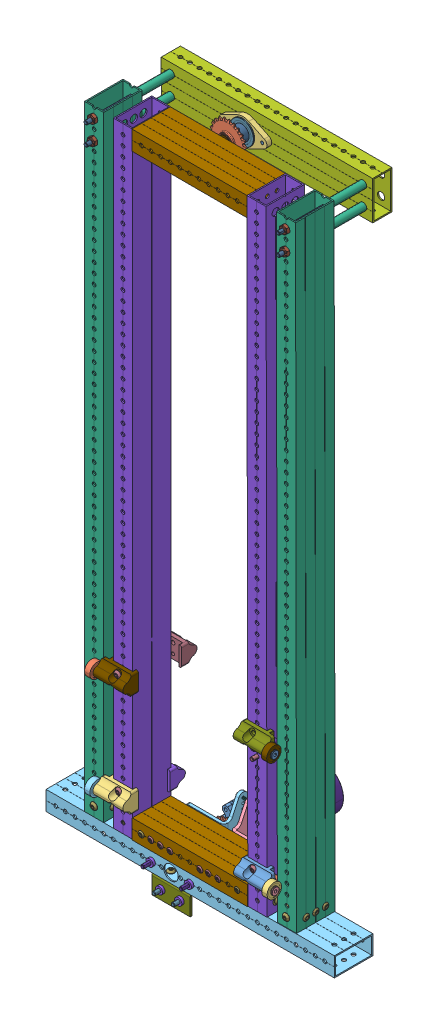
SolidWorks assembly WCP - GreyT Elevator (Cascade, 1 Stage).step, configuration Default. Lengths in mm.
Overall size (381 869.61 219.47).
186 component instances, 76 part files, 114 mates.
Components (placement in the parent):
- WCP-0323 - Elevator Clamping Block^WCP - GreyT Elevator (Cascade, 1 Stage).step-1: WCP-0323 - Elevator Clamping Block^WCP - GreyT Elevator (Cascade, 1 Stage).step [Default] at (101.6635 57.15 25.4) x (0 0 -1) z (1 0 0) size (29.22 25.41 49.35) (virtual)
  - WCP-0323-001 Rev2(7)^WCP-0323 - Elevator Clamping Block_WCP - GreyT Elevator (Cascade, 1 Stage).step-1: WCP-0323-001 Rev2(7)^WCP-0323 - Elevator Clamping Block_WCP - GreyT Elevator (Cascade, 1 Stage).step [Default] at origin size (20.38 25.41 40.49) (virtual)
  - WCP-0498 Rev1(7)^WCP-0323 - Elevator Clamping Block_WCP - GreyT Elevator (Cascade, 1 Stage).step-1: WCP-0498 Rev1(7)^WCP-0323 - Elevator Clamping Block_WCP - GreyT Elevator (Cascade, 1 Stage).step [Default] at (2.254 0 6.7) x (0 0.307359 0.951594) z (-1 0 0) size (12 12 4) (virtual)
  - WCP-0212_0_250_radial_bearing(7)^WCP-0323 - Elevator Clamping Block_WCP - GreyT Elevator (Cascade, 1 Stage).step-1: WCP-0212_0_250_radial_bearing(7)^WCP-0323 - Elevator Clamping Block_WCP - GreyT Elevator (Cascade, 1 Stage).step [Default] at (-9.525 0 15.4781) size (19.05 19.05 7.14) (virtual)
  - WCP-0473 Rev1(7)^WCP-0323 - Elevator Clamping Block_WCP - GreyT Elevator (Cascade, 1 Stage).step-1: WCP-0473 Rev1(7)^WCP-0323 - Elevator Clamping Block_WCP - GreyT Elevator (Cascade, 1 Stage).step [Default] at (-9.525 0 10.4394) x (-0.082744 -0.996571 0) z (-0.996571 0.082744 0) size (9.53 20.65 9.53) (virtual)
  - #8-32 x .25L BHCS(7)^WCP-0323 - Elevator Clamping Block_WCP - GreyT Elevator (Cascade, 1 Stage).step-1: #8-32 x .25L BHCS(7)^WCP-0323 - Elevator Clamping Block_WCP - GreyT Elevator (Cascade, 1 Stage).step [Default] at (6.7178 0 6.7) x (0 -0.337236 -0.94142) z (1 0 0) size (10.28 8 12.02) (virtual)
- WCP-0323 - Elevator Clamping Block-1^WCP - GreyT Elevator (Cascade, 1 Stage).step-1: WCP-0323 - Elevator Clamping Block-1^WCP - GreyT Elevator (Cascade, 1 Stage).step [Default] at (101.6635 57.15 -25.4) x (0 0 1) z (1 0 0) size (29.22 25.41 49.35) (virtual)
  - WCP-0323-001 Rev2(4)^WCP-0323 - Elevator Clamping Block-1_WCP - GreyT Elevator (Cascade, 1 Stage).step-1: WCP-0323-001 Rev2(4)^WCP-0323 - Elevator Clamping Block-1_WCP - GreyT Elevator (Cascade, 1 Stage).step [Default] at origin size (20.38 25.41 40.49) (virtual)
  - WCP-0498 Rev1(4)^WCP-0323 - Elevator Clamping Block-1_WCP - GreyT Elevator (Cascade, 1 Stage).step-1: WCP-0498 Rev1(4)^WCP-0323 - Elevator Clamping Block-1_WCP - GreyT Elevator (Cascade, 1 Stage).step [Default] at (2.254 0 6.7) x (0 0.307359 0.951594) z (-1 0 0) size (12 12 4) (virtual)
  - WCP-0212_0_250_radial_bearing(4)^WCP-0323 - Elevator Clamping Block-1_WCP - GreyT Elevator (Cascade, 1 Stage).step-1: WCP-0212_0_250_radial_bearing(4)^WCP-0323 - Elevator Clamping Block-1_WCP - GreyT Elevator (Cascade, 1 Stage).step [Default] at (-9.525 0 15.4781) size (19.05 19.05 7.14) (virtual)
  - WCP-0473 Rev1(4)^WCP-0323 - Elevator Clamping Block-1_WCP - GreyT Elevator (Cascade, 1 Stage).step-1: WCP-0473 Rev1(4)^WCP-0323 - Elevator Clamping Block-1_WCP - GreyT Elevator (Cascade, 1 Stage).step [Default] at (-9.525 0 10.4394) x (-0.082744 -0.996571 0) z (-0.996571 0.082744 0) size (9.53 20.65 9.53) (virtual)
  - #8-32 x .25L BHCS(4)^WCP-0323 - Elevator Clamping Block-1_WCP - GreyT Elevator (Cascade, 1 Stage).step-1: #8-32 x .25L BHCS(4)^WCP-0323 - Elevator Clamping Block-1_WCP - GreyT Elevator (Cascade, 1 Stage).step [Default] at (6.7178 0 6.7) x (0 -0.337236 -0.94142) z (1 0 0) size (10.28 8 12.02) (virtual)
- WCP-0323 - Elevator Clamping Block-2^WCP - GreyT Elevator (Cascade, 1 Stage).step-1: WCP-0323 - Elevator Clamping Block-2^WCP - GreyT Elevator (Cascade, 1 Stage).step [Default] at (101.6635 196.85 -25.4) x (0 0 1) z (1 0 0) size (29.22 25.41 49.35) (virtual)
  - WCP-0323-001 Rev2^WCP-0323 - Elevator Clamping Block-2_WCP - GreyT Elevator (Cascade, 1 Stage).step-1: WCP-0323-001 Rev2^WCP-0323 - Elevator Clamping Block-2_WCP - GreyT Elevator (Cascade, 1 Stage).step [Default] at origin size (20.38 25.41 40.49) (virtual)
  - WCP-0498 Rev1^WCP-0323 - Elevator Clamping Block-2_WCP - GreyT Elevator (Cascade, 1 Stage).step-1: WCP-0498 Rev1^WCP-0323 - Elevator Clamping Block-2_WCP - GreyT Elevator (Cascade, 1 Stage).step [Default] at (2.254 0 6.7) x (0 0.307359 0.951594) z (-1 0 0) size (12 12 4) (virtual)
  - WCP-0212_0_250_radial_bearing^WCP-0323 - Elevator Clamping Block-2_WCP - GreyT Elevator (Cascade, 1 Stage).step-1: WCP-0212_0_250_radial_bearing^WCP-0323 - Elevator Clamping Block-2_WCP - GreyT Elevator (Cascade, 1 Stage).step [Default] at (-9.525 0 15.4781) size (19.05 19.05 7.14) (virtual)
  - WCP-0473 Rev1^WCP-0323 - Elevator Clamping Block-2_WCP - GreyT Elevator (Cascade, 1 Stage).step-1: WCP-0473 Rev1^WCP-0323 - Elevator Clamping Block-2_WCP - GreyT Elevator (Cascade, 1 Stage).step [Default] at (-9.525 0 10.4394) x (-0.082744 -0.996571 0) z (-0.996571 0.082744 0) size (9.53 20.65 9.53) (virtual)
  - #8-32 x .25L BHCS^WCP-0323 - Elevator Clamping Block-2_WCP - GreyT Elevator (Cascade, 1 Stage).step-1: #8-32 x .25L BHCS^WCP-0323 - Elevator Clamping Block-2_WCP - GreyT Elevator (Cascade, 1 Stage).step [Default] at (6.7178 0 6.7) x (0 -0.337236 -0.94142) z (1 0 0) size (10.28 8 12.02) (virtual)
- WCP-0323 - Elevator Clamping Block-3^WCP - GreyT Elevator (Cascade, 1 Stage).step-1: WCP-0323 - Elevator Clamping Block-3^WCP - GreyT Elevator (Cascade, 1 Stage).step [Default] at (102.2013 214.1019 26.4322) x (0.002419 0.000009 -0.999997) z (0.999996 0.001569 0.002419) size (29.22 25.41 49.35) (virtual)
  - WCP-0323-001 Rev2(8)^WCP-0323 - Elevator Clamping Block-3_WCP - GreyT Elevator (Cascade, 1 Stage).step-1: WCP-0323-001 Rev2(8)^WCP-0323 - Elevator Clamping Block-3_WCP - GreyT Elevator (Cascade, 1 Stage).step [Default] at origin size (20.38 25.41 40.49) (virtual)
  - WCP-0498 Rev1(8)^WCP-0323 - Elevator Clamping Block-3_WCP - GreyT Elevator (Cascade, 1 Stage).step-1: WCP-0498 Rev1(8)^WCP-0323 - Elevator Clamping Block-3_WCP - GreyT Elevator (Cascade, 1 Stage).step [Default] at (2.254 0 6.7) x (0 0.307359 0.951594) z (-1 0 0) size (12 12 4) (virtual)
  - WCP-0212_0_250_radial_bearing(8)^WCP-0323 - Elevator Clamping Block-3_WCP - GreyT Elevator (Cascade, 1 Stage).step-1: WCP-0212_0_250_radial_bearing(8)^WCP-0323 - Elevator Clamping Block-3_WCP - GreyT Elevator (Cascade, 1 Stage).step [Default] at (-9.525 0 15.4781) size (19.05 19.05 7.14) (virtual)
  - WCP-0473 Rev1(8)^WCP-0323 - Elevator Clamping Block-3_WCP - GreyT Elevator (Cascade, 1 Stage).step-1: WCP-0473 Rev1(8)^WCP-0323 - Elevator Clamping Block-3_WCP - GreyT Elevator (Cascade, 1 Stage).step [Default] at (-9.525 0 10.4394) x (-0.082744 -0.996571 0) z (-0.996571 0.082744 0) size (9.53 20.65 9.53) (virtual)
  - #8-32 x .25L BHCS(8)^WCP-0323 - Elevator Clamping Block-3_WCP - GreyT Elevator (Cascade, 1 Stage).step-1: #8-32 x .25L BHCS(8)^WCP-0323 - Elevator Clamping Block-3_WCP - GreyT Elevator (Cascade, 1 Stage).step [Default] at (6.7178 0 6.7) x (0 -0.337236 -0.94142) z (1 0 0) size (10.28 8 12.02) (virtual)
- WCP-0323 - Elevator Clamping Block-4^WCP - GreyT Elevator (Cascade, 1 Stage).step-1: WCP-0323 - Elevator Clamping Block-4^WCP - GreyT Elevator (Cascade, 1 Stage).step [Default] at (-101.6635 57.15 25.4) x (0 0 -1) z (-1 0 0) size (29.22 25.41 49.35) (virtual)
  - WCP-0323-001 Rev2(5)^WCP-0323 - Elevator Clamping Block-4_WCP - GreyT Elevator (Cascade, 1 Stage).step-1: WCP-0323-001 Rev2(5)^WCP-0323 - Elevator Clamping Block-4_WCP - GreyT Elevator (Cascade, 1 Stage).step [Default] at origin size (20.38 25.41 40.49) (virtual)
  - WCP-0498 Rev1(5)^WCP-0323 - Elevator Clamping Block-4_WCP - GreyT Elevator (Cascade, 1 Stage).step-1: WCP-0498 Rev1(5)^WCP-0323 - Elevator Clamping Block-4_WCP - GreyT Elevator (Cascade, 1 Stage).step [Default] at (2.254 0 6.7) x (0 0.307359 0.951594) z (-1 0 0) size (12 12 4) (virtual)
  - WCP-0212_0_250_radial_bearing(5)^WCP-0323 - Elevator Clamping Block-4_WCP - GreyT Elevator (Cascade, 1 Stage).step-1: WCP-0212_0_250_radial_bearing(5)^WCP-0323 - Elevator Clamping Block-4_WCP - GreyT Elevator (Cascade, 1 Stage).step [Default] at (-9.525 0 15.4781) size (19.05 19.05 7.14) (virtual)
  - WCP-0473 Rev1(5)^WCP-0323 - Elevator Clamping Block-4_WCP - GreyT Elevator (Cascade, 1 Stage).step-1: WCP-0473 Rev1(5)^WCP-0323 - Elevator Clamping Block-4_WCP - GreyT Elevator (Cascade, 1 Stage).step [Default] at (-9.525 0 10.4394) x (-0.082744 -0.996571 0) z (-0.996571 0.082744 0) size (9.53 20.65 9.53) (virtual)
  - #8-32 x .25L BHCS(5)^WCP-0323 - Elevator Clamping Block-4_WCP - GreyT Elevator (Cascade, 1 Stage).step-1: #8-32 x .25L BHCS(5)^WCP-0323 - Elevator Clamping Block-4_WCP - GreyT Elevator (Cascade, 1 Stage).step [Default] at (6.7178 0 6.7) x (0 -0.337236 -0.94142) z (1 0 0) size (10.28 8 12.02) (virtual)
- WCP-0323 - Elevator Clamping Block-5^WCP - GreyT Elevator (Cascade, 1 Stage).step-1: WCP-0323 - Elevator Clamping Block-5^WCP - GreyT Elevator (Cascade, 1 Stage).step [Default] at (-101.6635 57.15 -25.4) x (0 0 1) z (-1 0 0) size (29.22 25.41 49.35) (virtual)
  - WCP-0323-001 Rev2(2)^WCP-0323 - Elevator Clamping Block-5_WCP - GreyT Elevator (Cascade, 1 Stage).step-1: WCP-0323-001 Rev2(2)^WCP-0323 - Elevator Clamping Block-5_WCP - GreyT Elevator (Cascade, 1 Stage).step [Default] at origin size (20.38 25.41 40.49) (virtual)
  - WCP-0498 Rev1(2)^WCP-0323 - Elevator Clamping Block-5_WCP - GreyT Elevator (Cascade, 1 Stage).step-1: WCP-0498 Rev1(2)^WCP-0323 - Elevator Clamping Block-5_WCP - GreyT Elevator (Cascade, 1 Stage).step [Default] at (2.254 0 6.7) x (0 0.307359 0.951594) z (-1 0 0) size (12 12 4) (virtual)
  - WCP-0212_0_250_radial_bearing(2)^WCP-0323 - Elevator Clamping Block-5_WCP - GreyT Elevator (Cascade, 1 Stage).step-1: WCP-0212_0_250_radial_bearing(2)^WCP-0323 - Elevator Clamping Block-5_WCP - GreyT Elevator (Cascade, 1 Stage).step [Default] at (-9.525 0 15.4781) size (19.05 19.05 7.14) (virtual)
  - WCP-0473 Rev1(2)^WCP-0323 - Elevator Clamping Block-5_WCP - GreyT Elevator (Cascade, 1 Stage).step-1: WCP-0473 Rev1(2)^WCP-0323 - Elevator Clamping Block-5_WCP - GreyT Elevator (Cascade, 1 Stage).step [Default] at (-9.525 0 10.4394) x (-0.082744 -0.996571 0) z (-0.996571 0.082744 0) size (9.53 20.65 9.53) (virtual)
  - #8-32 x .25L BHCS(2)^WCP-0323 - Elevator Clamping Block-5_WCP - GreyT Elevator (Cascade, 1 Stage).step-1: #8-32 x .25L BHCS(2)^WCP-0323 - Elevator Clamping Block-5_WCP - GreyT Elevator (Cascade, 1 Stage).step [Default] at (6.7178 0 6.7) x (0 -0.337236 -0.94142) z (1 0 0) size (10.28 8 12.02) (virtual)
- WCP-0323 - Elevator Clamping Block-6^WCP - GreyT Elevator (Cascade, 1 Stage).step-1: WCP-0323 - Elevator Clamping Block-6^WCP - GreyT Elevator (Cascade, 1 Stage).step [Default] at (-101.6 192.0731 -40.688) x (0 0 1) z (-1 0 0) size (29.22 25.41 49.35) (virtual)
  - WCP-0323-001 Rev2(3)^WCP-0323 - Elevator Clamping Block-6_WCP - GreyT Elevator (Cascade, 1 Stage).step-1: WCP-0323-001 Rev2(3)^WCP-0323 - Elevator Clamping Block-6_WCP - GreyT Elevator (Cascade, 1 Stage).step [Default] at origin size (20.38 25.41 40.49) (virtual)
  - WCP-0498 Rev1(3)^WCP-0323 - Elevator Clamping Block-6_WCP - GreyT Elevator (Cascade, 1 Stage).step-1: WCP-0498 Rev1(3)^WCP-0323 - Elevator Clamping Block-6_WCP - GreyT Elevator (Cascade, 1 Stage).step [Default] at (2.254 0 6.7) x (0 0.307359 0.951594) z (-1 0 0) size (12 12 4) (virtual)
  - WCP-0212_0_250_radial_bearing(3)^WCP-0323 - Elevator Clamping Block-6_WCP - GreyT Elevator (Cascade, 1 Stage).step-1: WCP-0212_0_250_radial_bearing(3)^WCP-0323 - Elevator Clamping Block-6_WCP - GreyT Elevator (Cascade, 1 Stage).step [Default] at (-9.525 0 15.4781) size (19.05 19.05 7.14) (virtual)
  - WCP-0473 Rev1(3)^WCP-0323 - Elevator Clamping Block-6_WCP - GreyT Elevator (Cascade, 1 Stage).step-1: WCP-0473 Rev1(3)^WCP-0323 - Elevator Clamping Block-6_WCP - GreyT Elevator (Cascade, 1 Stage).step [Default] at (-9.525 0 10.4394) x (-0.082744 -0.996571 0) z (-0.996571 0.082744 0) size (9.53 20.65 9.53) (virtual)
  - #8-32 x .25L BHCS(3)^WCP-0323 - Elevator Clamping Block-6_WCP - GreyT Elevator (Cascade, 1 Stage).step-1: #8-32 x .25L BHCS(3)^WCP-0323 - Elevator Clamping Block-6_WCP - GreyT Elevator (Cascade, 1 Stage).step [Default] at (6.7178 0 6.7) x (0 -0.337236 -0.94142) z (1 0 0) size (10.28 8 12.02) (virtual)
- WCP-0323 - Elevator Clamping Block-7^WCP - GreyT Elevator (Cascade, 1 Stage).step-1: WCP-0323 - Elevator Clamping Block-7^WCP - GreyT Elevator (Cascade, 1 Stage).step [Default] at (-101.6 192.0731 25.4) x (0 0 -1) z (-1 0 0) size (29.22 25.41 49.35) (virtual)
  - WCP-0323-001 Rev2(6)^WCP-0323 - Elevator Clamping Block-7_WCP - GreyT Elevator (Cascade, 1 Stage).step-1: WCP-0323-001 Rev2(6)^WCP-0323 - Elevator Clamping Block-7_WCP - GreyT Elevator (Cascade, 1 Stage).step [Default] at origin size (20.38 25.41 40.49) (virtual)
  - WCP-0498 Rev1(6)^WCP-0323 - Elevator Clamping Block-7_WCP - GreyT Elevator (Cascade, 1 Stage).step-1: WCP-0498 Rev1(6)^WCP-0323 - Elevator Clamping Block-7_WCP - GreyT Elevator (Cascade, 1 Stage).step [Default] at (2.254 0 6.7) x (0 0.307359 0.951594) z (-1 0 0) size (12 12 4) (virtual)
  - WCP-0212_0_250_radial_bearing(6)^WCP-0323 - Elevator Clamping Block-7_WCP - GreyT Elevator (Cascade, 1 Stage).step-1: WCP-0212_0_250_radial_bearing(6)^WCP-0323 - Elevator Clamping Block-7_WCP - GreyT Elevator (Cascade, 1 Stage).step [Default] at (-9.525 0 15.4781) size (19.05 19.05 7.14) (virtual)
  - WCP-0473 Rev1(6)^WCP-0323 - Elevator Clamping Block-7_WCP - GreyT Elevator (Cascade, 1 Stage).step-1: WCP-0473 Rev1(6)^WCP-0323 - Elevator Clamping Block-7_WCP - GreyT Elevator (Cascade, 1 Stage).step [Default] at (-9.525 0 10.4394) x (-0.082744 -0.996571 0) z (-0.996571 0.082744 0) size (9.53 20.65 9.53) (virtual)
  - #8-32 x .25L BHCS(6)^WCP-0323 - Elevator Clamping Block-7_WCP - GreyT Elevator (Cascade, 1 Stage).step-1: #8-32 x .25L BHCS(6)^WCP-0323 - Elevator Clamping Block-7_WCP - GreyT Elevator (Cascade, 1 Stage).step [Default] at (6.7178 0 6.7) x (0 -0.337236 -0.94142) z (1 0 0) size (10.28 8 12.02) (virtual)
- WCP-EX-0018-001^WCP - GreyT Elevator (Cascade, 1 Stage).step-1: WCP-EX-0018-001^WCP - GreyT Elevator (Cascade, 1 Stage).step [Default] x (1 0 0) z (0 -1 0) size (381 50.8 25.4) (virtual)
- WCP-EX-0018-005^WCP - GreyT Elevator (Cascade, 1 Stage).step-1: WCP-EX-0018-005^WCP - GreyT Elevator (Cascade, 1 Stage).step [Default] at (127.0437 610.2494 0.0748) x (0.001569 -0.999999 -0.000005) z (0.999996 0.001569 0.002419) size (812.8 50.8 25.4) (virtual)
- WCP-EX-0018-002^WCP - GreyT Elevator (Cascade, 1 Stage).step-1: WCP-EX-0018-002^WCP - GreyT Elevator (Cascade, 1 Stage).step [Default] at (0.0319 800.4229 -88.6828) x (0.999997 0.002542 0) z (0 0 1) size (279.4 50.8 25.4) (virtual)
- WCP-EX-0018-003^WCP - GreyT Elevator (Cascade, 1 Stage).step-1: WCP-EX-0018-003^WCP - GreyT Elevator (Cascade, 1 Stage).step [Default] at (88.782 711.7895 1.0039) x (0.001569 -0.999999 -0.000005) z (-0.999996 -0.001569 -0.002419) size (812.8 50.8 25.4) (virtual)
- WCP-EX-0018-004^WCP - GreyT Elevator (Cascade, 1 Stage).step-1: WCP-EX-0018-004^WCP - GreyT Elevator (Cascade, 1 Stage).step [Default] at (0.9567 25.7475 1.5065) x (0.999996 0.001569 0.002419) z (0.001569 -0.999999 0.000002) size (152.4 50.8 25.4) (virtual)
- WCP-EX-0018-004^WCP - GreyT Elevator (Cascade, 1 Stage).step-2: WCP-EX-0018-004^WCP - GreyT Elevator (Cascade, 1 Stage).step [Default] at (-0.277 813.2499 0.7893) x (0.999996 0.001569 0.002419) z (-0.001569 0.999999 0.000005) size (152.4 50.8 25.4) (virtual)
- WCP-EX-0018-005^WCP - GreyT Elevator (Cascade, 1 Stage).step-2: WCP-EX-0018-005^WCP - GreyT Elevator (Cascade, 1 Stage).step [Default] at (-127 609.6 0) x (0 -1 0) z (1 0 0) size (812.8 50.8 25.4) (virtual)
- 10-32 SHCS - No Thread_WCP-0274 - 4.500^WCP - GreyT Elevator (Cascade, 1 Stage).step-1: 10-32 SHCS - No Thread_WCP-0274 - 4.500^WCP - GreyT Elevator (Cascade, 1 Stage).step [Default] at (127.0637 788.0458 -77.5703) x (0.451844 0.892097 0) z (-0.892097 0.451844 0) size (7.67 119.13 7.67) (virtual)
- 10-32 SHCS - No Thread_WCP-0274 - 4.500^WCP - GreyT Elevator (Cascade, 1 Stage).step-2: 10-32 SHCS - No Thread_WCP-0274 - 4.500^WCP - GreyT Elevator (Cascade, 1 Stage).step [Default] at (126.9992 813.4457 -77.5703) x (0.495006 -0.86889 0) z (0.86889 0.495006 0) size (7.67 119.13 7.67) (virtual)
- WCP-0326 Rev1^WCP - GreyT Elevator (Cascade, 1 Stage).step-1: WCP-0326 Rev1^WCP - GreyT Elevator (Cascade, 1 Stage).step [Default] at (127.0637 788.0458 27.9921) x (-0.023206 0.999731 0) z (0.999731 0.023206 0) size (11.02 4.76 11) (virtual)
- WCP-0326 Rev1^WCP - GreyT Elevator (Cascade, 1 Stage).step-2: WCP-0326 Rev1^WCP - GreyT Elevator (Cascade, 1 Stage).step [Default] at (126.9992 813.4457 27.9921) x (-0.196323 0.980539 0) z (0.980539 0.196323 0) size (11.02 4.76 11) (virtual)
- 10-32 BHCS - No Thread_WCP-0252 - 0.375^WCP - GreyT Elevator (Cascade, 1 Stage).step-1: 10-32 BHCS - No Thread_WCP-0252 - 0.375^WCP - GreyT Elevator (Cascade, 1 Stage).step [Default] at (127 11.1125 12.7) x (0.583861 0 0.811854) z (0.811854 0 -0.583861) size (9.17 12.1 9.17) (virtual)
- 10-32 BHCS - No Thread_WCP-0252 - 0.375^WCP - GreyT Elevator (Cascade, 1 Stage).step-2: 10-32 BHCS - No Thread_WCP-0252 - 0.375^WCP - GreyT Elevator (Cascade, 1 Stage).step [Default] at (127 11.1125 0) x (0.583861 0 0.811854) z (0.811854 0 -0.583861) size (9.17 12.1 9.17) (virtual)
- 10-32 BHCS - No Thread_WCP-0252 - 0.375^WCP - GreyT Elevator (Cascade, 1 Stage).step-3: 10-32 BHCS - No Thread_WCP-0252 - 0.375^WCP - GreyT Elevator (Cascade, 1 Stage).step [Default] at (127 11.1125 -12.7) x (0.583861 0 0.811854) z (0.811854 0 -0.583861) size (9.17 12.1 9.17) (virtual)
- 10-32 BHCS - No Thread_WCP-0252 - 0.375^WCP - GreyT Elevator (Cascade, 1 Stage).step-4: 10-32 BHCS - No Thread_WCP-0252 - 0.375^WCP - GreyT Elevator (Cascade, 1 Stage).step [Default] at (139.7 25.4 12.7) x (0 -0.948064 0.318079) z (0 0.318079 0.948064) size (9.17 12.1 9.17) (virtual)
- 10-32 BHCS - No Thread_WCP-0252 - 0.375^WCP - GreyT Elevator (Cascade, 1 Stage).step-5: 10-32 BHCS - No Thread_WCP-0252 - 0.375^WCP - GreyT Elevator (Cascade, 1 Stage).step [Default] at (139.7 25.4 0) x (0 -0.948064 0.318079) z (0 0.318079 0.948064) size (9.17 12.1 9.17) (virtual)
- 10-32 BHCS - No Thread_WCP-0252 - 0.375^WCP - GreyT Elevator (Cascade, 1 Stage).step-6: 10-32 BHCS - No Thread_WCP-0252 - 0.375^WCP - GreyT Elevator (Cascade, 1 Stage).step [Default] at (139.7 25.4 -12.7) x (0 -0.948064 0.318079) z (0 0.318079 0.948064) size (9.17 12.1 9.17) (virtual)
- 10-32 BHCS - No Thread_WCP-0252 - 0.375^WCP - GreyT Elevator (Cascade, 1 Stage).step-7: 10-32 BHCS - No Thread_WCP-0252 - 0.375^WCP - GreyT Elevator (Cascade, 1 Stage).step [Default] at (114.3 25.4 12.7) x (0 -0.983057 -0.183299) z (0 0.183299 -0.983057) size (9.17 12.1 9.17) (virtual)
- 10-32 BHCS - No Thread_WCP-0252 - 0.375^WCP - GreyT Elevator (Cascade, 1 Stage).step-8: 10-32 BHCS - No Thread_WCP-0252 - 0.375^WCP - GreyT Elevator (Cascade, 1 Stage).step [Default] at (114.3 25.4 0) x (0 -0.639879 0.768476) z (0 -0.768476 -0.639879) size (9.17 12.1 9.17) (virtual)
- 10-32 BHCS - No Thread_WCP-0252 - 0.375^WCP - GreyT Elevator (Cascade, 1 Stage).step-9: 10-32 BHCS - No Thread_WCP-0252 - 0.375^WCP - GreyT Elevator (Cascade, 1 Stage).step [Default] at (114.3 25.4 -12.7) x (0 -0.639879 0.768476) z (0 -0.768476 -0.639879) size (9.17 12.1 9.17) (virtual)
- 10-32 BHCS - No Thread_WCP-0261 - 2.500^WCP - GreyT Elevator (Cascade, 1 Stage).step-1: 10-32 BHCS - No Thread_WCP-0261 - 2.500^WCP - GreyT Elevator (Cascade, 1 Stage).step [Default] at (38.1 25.4 25.4) x (-0.574084 -0.818796 0) z (-0.818796 0.574084 0) size (9.17 66.07 9.17) (virtual)
- 10-32 BHCS - No Thread_WCP-0261 - 2.500^WCP - GreyT Elevator (Cascade, 1 Stage).step-2: 10-32 BHCS - No Thread_WCP-0261 - 2.500^WCP - GreyT Elevator (Cascade, 1 Stage).step [Default] at (-50.8 25.4 25.4) x (-0.574084 -0.818796 0) z (-0.818796 0.574084 0) size (9.17 66.07 9.17) (virtual)
- 10-32 BHCS - No Thread_WCP-0261 - 2.500^WCP - GreyT Elevator (Cascade, 1 Stage).step-3: 10-32 BHCS - No Thread_WCP-0261 - 2.500^WCP - GreyT Elevator (Cascade, 1 Stage).step [Default] at (-38.1 25.4 25.4) x (-0.574084 -0.818796 0) z (-0.818796 0.574084 0) size (9.17 66.07 9.17) (virtual)
- 10-32 BHCS - No Thread_WCP-0261 - 2.500^WCP - GreyT Elevator (Cascade, 1 Stage).step-4: 10-32 BHCS - No Thread_WCP-0261 - 2.500^WCP - GreyT Elevator (Cascade, 1 Stage).step [Default] at (-25.4 25.4 25.4) x (-0.574084 -0.818796 0) z (-0.818796 0.574084 0) size (9.17 66.07 9.17) (virtual)
- WCP-0326 Rev1^WCP - GreyT Elevator (Cascade, 1 Stage).step-3: WCP-0326 Rev1^WCP - GreyT Elevator (Cascade, 1 Stage).step [Default] at (38.1 25.4 -31.7749) x (-0.969621 0.244611 0) z (-0.244611 -0.969621 0) size (11.02 4.76 11) (virtual)
- WCP-0326 Rev1^WCP - GreyT Elevator (Cascade, 1 Stage).step-4: WCP-0326 Rev1^WCP - GreyT Elevator (Cascade, 1 Stage).step [Default] at (14.3113 24.2689 -31.7749) x (-0.281999 0.959415 0) z (-0.959415 -0.281999 0) size (11.02 4.76 11) (virtual)
- WCP-0326 Rev1^WCP - GreyT Elevator (Cascade, 1 Stage).step-5: WCP-0326 Rev1^WCP - GreyT Elevator (Cascade, 1 Stage).step [Default] at (-25.4 25.4 -31.7749) x (-0.281999 0.959415 0) z (-0.959415 -0.281999 0) size (11.02 4.76 11) (virtual)
- WCP-0326 Rev1^WCP - GreyT Elevator (Cascade, 1 Stage).step-6: WCP-0326 Rev1^WCP - GreyT Elevator (Cascade, 1 Stage).step [Default] at (-38.1 25.4 -31.7749) x (-0.281999 0.959415 0) z (-0.959415 -0.281999 0) size (11.02 4.76 11) (virtual)
- WCP-0326 Rev1^WCP - GreyT Elevator (Cascade, 1 Stage).step-7: WCP-0326 Rev1^WCP - GreyT Elevator (Cascade, 1 Stage).step [Default] at (-50.8 25.4 -31.7749) x (-0.281999 0.959415 0) z (-0.959415 -0.281999 0) size (11.02 4.76 11) (virtual)
- WCP-0326 Rev1^WCP - GreyT Elevator (Cascade, 1 Stage).step-8: WCP-0326 Rev1^WCP - GreyT Elevator (Cascade, 1 Stage).step [Default] at (25.4 25.4 -31.7749) x (-0.281999 0.959415 0) z (-0.959415 -0.281999 0) size (11.02 4.76 11) (virtual)
- 10-32 BHCS - No Thread_WCP-0253 - 0.500.step-1: 10-32 BHCS - No Thread_WCP-0253 - 0.500.step [Default] at (-38.1 -25.4 23.114) x (0.466097 -0.884734 0) z (0.884734 0.466097 0) size (9.17 15.27 9.17)
- 10-32 BHCS - No Thread_WCP-0253 - 0.500.step-2: 10-32 BHCS - No Thread_WCP-0253 - 0.500.step [Default] at (-12.7 -25.4 23.114) x (-0.99286 -0.119284 0) z (0.119284 -0.99286 0) size (9.17 15.27 9.17)
- 10-32 BHCS - No Thread_WCP-0252 - 0.375^WCP - GreyT Elevator (Cascade, 1 Stage).step-10: 10-32 BHCS - No Thread_WCP-0252 - 0.375^WCP - GreyT Elevator (Cascade, 1 Stage).step [Default] at (-12.7 -11.1125 12.7) x (0.458328 0 0.888783) z (-0.888783 0 0.458328) size (9.17 12.1 9.17) (virtual)
- 10-32 BHCS - No Thread_WCP-0252 - 0.375^WCP - GreyT Elevator (Cascade, 1 Stage).step-11: 10-32 BHCS - No Thread_WCP-0252 - 0.375^WCP - GreyT Elevator (Cascade, 1 Stage).step [Default] at (-38.1 -11.1125 12.7) x (0.458328 0 0.888783) z (-0.888783 0 0.458328) size (9.17 12.1 9.17) (virtual)
- WCP-0326 Rev1^WCP - GreyT Elevator (Cascade, 1 Stage).step-9: WCP-0326 Rev1^WCP - GreyT Elevator (Cascade, 1 Stage).step [Default] at (-12.7 -17.3609 12.7) x (-0.999719 0 -0.023694) z (-0.023694 0 0.999719) size (11.02 4.76 11) (virtual)
- WCP-0326 Rev1^WCP - GreyT Elevator (Cascade, 1 Stage).step-10: WCP-0326 Rev1^WCP - GreyT Elevator (Cascade, 1 Stage).step [Default] at (-38.1 -17.3609 12.7) x (-0.806355 0 -0.591432) z (-0.591432 0 0.806355) size (11.02 4.76 11) (virtual)
- 10-32 BHCS - No Thread_WCP-0252 - 0.375^WCP - GreyT Elevator (Cascade, 1 Stage).step-12: 10-32 BHCS - No Thread_WCP-0252 - 0.375^WCP - GreyT Elevator (Cascade, 1 Stage).step [Default] at (127 25.4 25.4) x (0.238233 -0.971208 0) z (-0.971208 -0.238233 0) size (9.17 12.1 9.17) (virtual)
- 10-32 BHCS - No Thread_WCP-0252 - 0.375^WCP - GreyT Elevator (Cascade, 1 Stage).step-13: 10-32 BHCS - No Thread_WCP-0252 - 0.375^WCP - GreyT Elevator (Cascade, 1 Stage).step [Default] at (127 25.4 -25.4) x (0.705419 -0.708791 0) z (0.708791 0.705419 0) size (9.17 12.1 9.17) (virtual)
- #4-40 x .750L SHCS^WCP - GreyT Elevator (Cascade, 1 Stage).step-1: #4-40 x .750L SHCS^WCP - GreyT Elevator (Cascade, 1 Stage).step [Default] at (-2.4913 57.15 -50.8) x (0 0.222099 -0.975024) z (1 0 0) size (4.65 4.65 21.9) (virtual)
- NFS-0016_#4-40_thin_locknut_Default_As Machined_^WCP - GreyT Elevator (Cascade, 1 Stage).step-1: NFS-0016_#4-40_thin_locknut_Default_As Machined_^WCP - GreyT Elevator (Cascade, 1 Stage).step [Default] at (-10.35 57.15 -50.8) x (0 0.495484 -0.868617) z (0 0.868617 0.495484) size (6.37 2.79 7.35) (virtual)
- #4-40 x .750L SHCS^WCP - GreyT Elevator (Cascade, 1 Stage).step-2: #4-40 x .750L SHCS^WCP - GreyT Elevator (Cascade, 1 Stage).step [Default] at (-2.4913 30.6189 -50.8) x (0 0.423366 0.905959) z (1 0 0) size (4.65 4.65 21.9) (virtual)
- #4-40 x .750L SHCS^WCP - GreyT Elevator (Cascade, 1 Stage).step-3: #4-40 x .750L SHCS^WCP - GreyT Elevator (Cascade, 1 Stage).step [Default] at (-2.4913 44.45 -50.8) x (0 -0.973772 0.227524) z (1 0 0) size (4.65 4.65 21.9) (virtual)
- NFS-0016_#4-40_thin_locknut_Default_As Machined_^WCP - GreyT Elevator (Cascade, 1 Stage).step-2: NFS-0016_#4-40_thin_locknut_Default_As Machined_^WCP - GreyT Elevator (Cascade, 1 Stage).step [Default] at (-10.35 44.45 -50.8) x (0 -0.910503 -0.413502) z (0 0.413502 -0.910503) size (6.37 2.79 7.35) (virtual)
- NFS-0016_#4-40_thin_locknut_Default_As Machined_^WCP - GreyT Elevator (Cascade, 1 Stage).step-3: NFS-0016_#4-40_thin_locknut_Default_As Machined_^WCP - GreyT Elevator (Cascade, 1 Stage).step [Default] at (-10.35 31.75 -50.8) x (0 0.495484 -0.868617) z (0 0.868617 0.495484) size (6.37 2.79 7.35) (virtual)
- 10-32 BHCS - No Thread_WCP-0261 - 2.500^WCP - GreyT Elevator (Cascade, 1 Stage).step-5: 10-32 BHCS - No Thread_WCP-0261 - 2.500^WCP - GreyT Elevator (Cascade, 1 Stage).step [Default] at (25.4 25.4 25.4) x (-0.574084 -0.818796 0) z (-0.818796 0.574084 0) size (9.17 66.07 9.17) (virtual)
- 10-32 BHCS - No Thread_WCP-0261 - 2.500^WCP - GreyT Elevator (Cascade, 1 Stage).step-6: 10-32 BHCS - No Thread_WCP-0261 - 2.500^WCP - GreyT Elevator (Cascade, 1 Stage).step [Default] at (14.3113 24.2689 25.5684) x (-0.574084 -0.818796 0) z (-0.818796 0.574084 0) size (9.17 66.07 9.17) (virtual)
- 10-32 BHCS - No Thread_WCP-0263 - 3.000^WCP - GreyT Elevator (Cascade, 1 Stage).step-1: 10-32 BHCS - No Thread_WCP-0263 - 3.000^WCP - GreyT Elevator (Cascade, 1 Stage).step [Default] at (0 0 -38.1) x (0.756715 -0.653745 0) z (0.653745 0.756715 0) size (9.17 78.77 9.17) (virtual)
- 10-32 BHCS - No Thread_WCP-0263 - 3.000^WCP - GreyT Elevator (Cascade, 1 Stage).step-2: 10-32 BHCS - No Thread_WCP-0263 - 3.000^WCP - GreyT Elevator (Cascade, 1 Stage).step [Default] at (-50.8 0 -38.1) x (0.756715 -0.653745 0) z (0.653745 0.756715 0) size (9.17 78.77 9.17) (virtual)
- WCP-0571 Rev1^WCP - GreyT Elevator (Cascade, 1 Stage).step-1: WCP-0571 Rev1^WCP - GreyT Elevator (Cascade, 1 Stage).step [Default] at (-25.3061 800.2094 -42.8231) size (15.88 15.88 15.71) (virtual)
- WCP-0571 Rev1^WCP - GreyT Elevator (Cascade, 1 Stage).step-2: WCP-0571 Rev1^WCP - GreyT Elevator (Cascade, 1 Stage).step [Default] at (-25.3061 800.2094 -112.3175) x (-0.990411 -0.138152 0) z (0 0 -1) size (15.88 15.88 15.71) (virtual)
- 10-32 BHCS - No Thread_WCP-0257 - 1.500.step-1: 10-32 BHCS - No Thread_WCP-0257 - 1.500.step [Default] at (0.0319 800.4229 -107.7328) x (-0.802481 0.596678 0) z (-0.596678 -0.802481 0) size (9.17 40.67 9.17)
- 10-32 BHCS - No Thread_WCP-0257 - 1.500.step-2: 10-32 BHCS - No Thread_WCP-0257 - 1.500.step [Default] at (-50.768 800.2938 -107.7328) x (-0.853188 0.521603 0) z (-0.521603 -0.853188 0) size (9.17 40.67 9.17)
- 10-32 BHCS - No Thread_WCP-0261 - 2.500^WCP - GreyT Elevator (Cascade, 1 Stage).step-7: 10-32 BHCS - No Thread_WCP-0261 - 2.500^WCP - GreyT Elevator (Cascade, 1 Stage).step [Default] at (88.9 63.5 30.1625) x (0.238233 -0.971208 0) z (-0.971208 -0.238233 0) size (9.17 66.07 9.17) (virtual)
- 10-32 BHCS - No Thread_WCP-0261 - 2.500^WCP - GreyT Elevator (Cascade, 1 Stage).step-8: 10-32 BHCS - No Thread_WCP-0261 - 2.500^WCP - GreyT Elevator (Cascade, 1 Stage).step [Default] at (88.9 50.8 -30.1625) x (0.035589 0.999367 0) z (-0.999367 0.035589 0) size (9.17 66.07 9.17) (virtual)
- 10-32 BHCS - No Thread_WCP-0261 - 2.500^WCP - GreyT Elevator (Cascade, 1 Stage).step-9: 10-32 BHCS - No Thread_WCP-0261 - 2.500^WCP - GreyT Elevator (Cascade, 1 Stage).step [Default] at (88.9 190.5 -30.1625) x (0.035589 0.999367 0) z (-0.999367 0.035589 0) size (9.17 66.07 9.17) (virtual)
- 10-32 BHCS - No Thread_WCP-0261 - 2.500^WCP - GreyT Elevator (Cascade, 1 Stage).step-10: 10-32 BHCS - No Thread_WCP-0261 - 2.500^WCP - GreyT Elevator (Cascade, 1 Stage).step [Default] at (88.9 203.2 30.1625) x (0.238233 -0.971208 0) z (-0.971208 -0.238233 0) size (9.17 66.07 9.17) (virtual)
- 10-32 BHCS - No Thread_WCP-0252 - 0.375^WCP - GreyT Elevator (Cascade, 1 Stage).step-14: 10-32 BHCS - No Thread_WCP-0252 - 0.375^WCP - GreyT Elevator (Cascade, 1 Stage).step [Default] at (77.7875 25.4 12.7) x (0 0.635714 0.771925) z (0 0.771925 -0.635714) size (9.17 12.1 9.17) (virtual)
- 10-32 BHCS - No Thread_WCP-0252 - 0.375^WCP - GreyT Elevator (Cascade, 1 Stage).step-15: 10-32 BHCS - No Thread_WCP-0252 - 0.375^WCP - GreyT Elevator (Cascade, 1 Stage).step [Default] at (77.7875 25.4 0) x (0 0.635714 0.771925) z (0 0.771925 -0.635714) size (9.17 12.1 9.17) (virtual)
- 10-32 BHCS - No Thread_WCP-0252 - 0.375^WCP - GreyT Elevator (Cascade, 1 Stage).step-16: 10-32 BHCS - No Thread_WCP-0252 - 0.375^WCP - GreyT Elevator (Cascade, 1 Stage).step [Default] at (77.7875 25.4 -12.7) x (0 0.635714 0.771925) z (0 0.771925 -0.635714) size (9.17 12.1 9.17) (virtual)
- 10-32 BHCS - No Thread_WCP-0252 - 0.375^WCP - GreyT Elevator (Cascade, 1 Stage).step-17: 10-32 BHCS - No Thread_WCP-0252 - 0.375^WCP - GreyT Elevator (Cascade, 1 Stage).step [Default] at (63.5 25.4 25.4) x (0.238233 -0.971208 0) z (-0.971208 -0.238233 0) size (9.17 12.1 9.17) (virtual)
- 10-32 BHCS - No Thread_WCP-0252 - 0.375^WCP - GreyT Elevator (Cascade, 1 Stage).step-18: 10-32 BHCS - No Thread_WCP-0252 - 0.375^WCP - GreyT Elevator (Cascade, 1 Stage).step [Default] at (63.5 25.4 -25.4) x (0.705419 -0.708791 0) z (0.708791 0.705419 0) size (9.17 12.1 9.17) (virtual)
- 10-32 BHCS - No Thread_WCP-0252 - 0.375^WCP - GreyT Elevator (Cascade, 1 Stage).step-19: 10-32 BHCS - No Thread_WCP-0252 - 0.375^WCP - GreyT Elevator (Cascade, 1 Stage).step [Default] at (102.4761 26.269 -0.7006) x (0 0.635714 0.771925) z (0 0.771925 -0.635714) size (9.17 12.1 9.17) (virtual)
- 10-32 BHCS - No Thread_WCP-0252 - 0.375^WCP - GreyT Elevator (Cascade, 1 Stage).step-20: 10-32 BHCS - No Thread_WCP-0252 - 0.375^WCP - GreyT Elevator (Cascade, 1 Stage).step [Default] at (102.4761 26.269 11.9994) x (0 0.635714 0.771925) z (0 0.771925 -0.635714) size (9.17 12.1 9.17) (virtual)
- 10-32 BHCS - No Thread_WCP-0252 - 0.375^WCP - GreyT Elevator (Cascade, 1 Stage).step-21: 10-32 BHCS - No Thread_WCP-0252 - 0.375^WCP - GreyT Elevator (Cascade, 1 Stage).step [Default] at (102.4761 26.269 -13.4006) x (0 0.635714 0.771925) z (0 0.771925 -0.635714) size (9.17 12.1 9.17) (virtual)
- WCP-0560 Rev1^WCP - GreyT Elevator (Cascade, 1 Stage).step-1: WCP-0560 Rev1^WCP - GreyT Elevator (Cascade, 1 Stage).step [Default] at (-25.4 0 -50.8) x (0.196104 0.980583 0) z (0 0 -1) size (47.96 47.68 9.53) (virtual)
- WCP-0560 Rev1^WCP - GreyT Elevator (Cascade, 1 Stage).step-2: WCP-0560 Rev1^WCP - GreyT Elevator (Cascade, 1 Stage).step [Default] at (-25.323 800.25 -50.5828) x (-0.92321 -0.384296 0) z (0 0 -1) size (47.96 47.68 9.53) (virtual)
- WCP-0476 Rev1^WCP - GreyT Elevator (Cascade, 1 Stage).step-1: WCP-0476 Rev1^WCP - GreyT Elevator (Cascade, 1 Stage).step [Default] at (-25.4 0 -34.925) size (63.5 34.92 6.35) (virtual)
- WCP-0476 Rev1^WCP - GreyT Elevator (Cascade, 1 Stage).step-2: WCP-0476 Rev1^WCP - GreyT Elevator (Cascade, 1 Stage).step [Default] at (-25.368 800.3583 -72.8078) x (0.999997 0.002542 0) z (0 0 1) size (63.5 34.92 6.35) (virtual)
- WCP-0476 Rev1^WCP - GreyT Elevator (Cascade, 1 Stage).step-3: WCP-0476 Rev1^WCP - GreyT Elevator (Cascade, 1 Stage).step [Default] at (-25.368 800.2938 -104.5578) size (63.5 34.92 6.35) (virtual)
- WCP-0583-025 Rev1_DefaultSM-FLAT-PATTERN^WCP - GreyT Elevator (Cascade, 1 Stage).step-1: WCP-0583-025 Rev1_DefaultSM-FLAT-PATTERN^WCP - GreyT Elevator (Cascade, 1 Stage).step [Default] at (23.8363 24.2689 -29.4) x (-1 0 0) z (0 0 -1) size (44.45 50.8 31.75) (virtual)
- WCP-0583-026 Rev1^WCP - GreyT Elevator (Cascade, 1 Stage).step-1: WCP-0583-026 Rev1^WCP - GreyT Elevator (Cascade, 1 Stage).step [Default] at (-31.75 25.4 -29.4) x (-1 0 0) z (0 0 -1) size (50.8 50.8 31.75) (virtual)
- WCP-0207 Rev1^WCP - GreyT Elevator (Cascade, 1 Stage).step-1: WCP-0207 Rev1^WCP - GreyT Elevator (Cascade, 1 Stage).step [Default] at (126.9992 813.4457 -50.5828) x (0 0 -1) z (0.999873 -0.015939 0) size (50.8 9.5 9.5) (virtual)
- WCP-0207 Rev1^WCP - GreyT Elevator (Cascade, 1 Stage).step-2: WCP-0207 Rev1^WCP - GreyT Elevator (Cascade, 1 Stage).step [Default] at (127.0637 788.0458 -50.5828) x (0 0 -1) z (0.999873 -0.015939 0) size (50.8 9.5 9.5) (virtual)
- WCP-0308 Rev1^WCP - GreyT Elevator (Cascade, 1 Stage).step-1: WCP-0308 Rev1^WCP - GreyT Elevator (Cascade, 1 Stage).step [Default] at (-50.8 0 -28.575) x (0 0 -1) z (0.995626 0.093431 0) size (6.35 9.5 9.5) (virtual)
- WCP-0308 Rev1^WCP - GreyT Elevator (Cascade, 1 Stage).step-2: WCP-0308 Rev1^WCP - GreyT Elevator (Cascade, 1 Stage).step [Default] at (0 0 -28.575) x (0 0 -1) z (0.995626 0.093431 0) size (6.35 9.5 9.5) (virtual)
- WCP-0307 Rev1^WCP - GreyT Elevator (Cascade, 1 Stage).step-1: WCP-0307 Rev1^WCP - GreyT Elevator (Cascade, 1 Stage).step [Default] at (-12.7 -25.4 26.9913) x (0 0 1) z (-0.952187 0.305516 0) size (3.18 9.5 9.5) (virtual)
- WCP-0307 Rev1^WCP - GreyT Elevator (Cascade, 1 Stage).step-2: WCP-0307 Rev1^WCP - GreyT Elevator (Cascade, 1 Stage).step [Default] at (-38.1 -25.4 26.9913) x (0 0 1) z (-0.952187 0.305516 0) size (3.18 9.5 9.5) (virtual)
- WCP-0307 Rev1^WCP - GreyT Elevator (Cascade, 1 Stage).step-3: WCP-0307 Rev1^WCP - GreyT Elevator (Cascade, 1 Stage).step [Default] at (0 0 26.9913) x (0 0 1) z (-0.952187 0.305516 0) size (3.18 9.5 9.5) (virtual)
- WCP-0307 Rev1^WCP - GreyT Elevator (Cascade, 1 Stage).step-4: WCP-0307 Rev1^WCP - GreyT Elevator (Cascade, 1 Stage).step [Default] at (-50.8 0 26.9913) x (0 0 1) z (-0.952187 0.305516 0) size (3.18 9.5 9.5) (virtual)
- WCP-0599 Rev1^WCP - GreyT Elevator (Cascade, 1 Stage).step-1: WCP-0599 Rev1^WCP - GreyT Elevator (Cascade, 1 Stage).step [Default] at (-25.3061 800.2094 -77.5703) x (0 0 -1) z (0.991671 -0.128795 0) size (63.5 12.67 13.72) (virtual)
- WCP-0790_500L_500_hex.step-1: WCP-0790_500L_500_hex.step [Default] at (-25.368 800.3583 -61.6953) x (0.991671 -0.128795 0) z (0 0 1) size (19.5 19.5 12.7)
- WCP-0789_250L_500_hex^WCP - GreyT Elevator (Cascade, 1 Stage).step-1: WCP-0789_250L_500_hex^WCP - GreyT Elevator (Cascade, 1 Stage).step [Default] at (-25.4 0 -42.8625) size (19.5 19.5 6.35) (virtual)
- WCP-0374 Rev1^WCP - GreyT Elevator (Cascade, 1 Stage).step-1: WCP-0374 Rev1^WCP - GreyT Elevator (Cascade, 1 Stage).step [Default] at (127 22.225 0) x (0 0 -1) z (1 0 0) size (44.07 19.05 18.67) (virtual)
- WCP-0379 Rev1^WCP - GreyT Elevator (Cascade, 1 Stage).step-1: WCP-0379 Rev1^WCP - GreyT Elevator (Cascade, 1 Stage).step [Default] at (127 22.225 0) x (0 0 -1) z (1 0 0) size (47.24 20.64 21.84) (virtual)
- WCP-0374 Rev1^WCP - GreyT Elevator (Cascade, 1 Stage).step-2: WCP-0374 Rev1^WCP - GreyT Elevator (Cascade, 1 Stage).step [Default] at (66.675 25.4 0) x (0 0 -1) z (0 1 0) size (44.07 19.05 18.67) (virtual)
- WCP-0379 Rev1^WCP - GreyT Elevator (Cascade, 1 Stage).step-2: WCP-0379 Rev1^WCP - GreyT Elevator (Cascade, 1 Stage).step [Default] at (66.675 25.4 0) x (0 0 -1) z (0 1 0) size (47.24 20.64 21.84) (virtual)
- WCP-0374 Rev1^WCP - GreyT Elevator (Cascade, 1 Stage).step-3: WCP-0374 Rev1^WCP - GreyT Elevator (Cascade, 1 Stage).step [Default] at (92.9511 26.269 -0.7006) x (0 0 -1) z (0 1 0) size (44.07 19.05 18.67) (virtual)
- WCP-0379 Rev1^WCP - GreyT Elevator (Cascade, 1 Stage).step-3: WCP-0379 Rev1^WCP - GreyT Elevator (Cascade, 1 Stage).step [Default] at (92.9511 26.142 -0.7006) x (0 0 -1) z (0 1 0) size (47.24 20.64 21.84) (virtual)
- WCP-0785_0_500_flanged_thunderhex_bearing.step-1: WCP-0785_0_500_flanged_thunderhex_bearing.step [Default] at (-25.4 0 -35.7188) x (-0.952019 0.30604 0) z (0 0 -1) size (31.12 31.12 7.94)
- WCP-0785_0_500_flanged_thunderhex_bearing.step-2: WCP-0785_0_500_flanged_thunderhex_bearing.step [Default] at (-25.368 800.2938 -105.3515) x (-0.914179 0.405311 0) z (0 0 -1) size (31.12 31.12 7.94)
- WCP-0785_0_500_flanged_thunderhex_bearing.step-3: WCP-0785_0_500_flanged_thunderhex_bearing.step [Default] at (-25.368 800.3583 -72.014) x (0.656952 0.753932 0) z (0 0 1) size (31.12 31.12 7.94)
- WCP-0800_500_hex_collar_high_strength^WCP - GreyT Elevator (Cascade, 1 Stage).step-1: WCP-0800_500_hex_collar_high_strength^WCP - GreyT Elevator (Cascade, 1 Stage).step [Default] at (-25.4 0 -60.325) x (0.520207 -0.85404 0) z (0 0 1) size (28.56 28.57 9.53) (virtual)
- WCP-0326 Rev1^WCP - GreyT Elevator (Cascade, 1 Stage).step-11: WCP-0326 Rev1^WCP - GreyT Elevator (Cascade, 1 Stage).step [Default] at (-127 812.8 27.7749) x (-0.127192 0.991878 0) z (0.991878 0.127192 0) size (11.02 4.76 11) (virtual)
- 10-32 SHCS - No Thread_WCP-0274 - 4.500^WCP - GreyT Elevator (Cascade, 1 Stage).step-3: 10-32 SHCS - No Thread_WCP-0274 - 4.500^WCP - GreyT Elevator (Cascade, 1 Stage).step [Default] at (-127 812.8 -77.5703) x (-0.495006 -0.86889 0) z (0.86889 -0.495006 0) size (7.67 119.13 7.67) (virtual)
- WCP-0326 Rev1^WCP - GreyT Elevator (Cascade, 1 Stage).step-12: WCP-0326 Rev1^WCP - GreyT Elevator (Cascade, 1 Stage).step [Default] at (-126.9354 787.4001 27.9921) x (0.023206 0.999731 0) z (0.999731 -0.023206 0) size (11.02 4.76 11) (virtual)
- 10-32 SHCS - No Thread_WCP-0274 - 4.500^WCP - GreyT Elevator (Cascade, 1 Stage).step-4: 10-32 SHCS - No Thread_WCP-0274 - 4.500^WCP - GreyT Elevator (Cascade, 1 Stage).step [Default] at (-126.9354 787.4001 -77.5703) x (-0.495006 -0.86889 0) z (0.86889 -0.495006 0) size (7.67 119.13 7.67) (virtual)
- 10-32 BHCS - No Thread_WCP-0252 - 0.375^WCP - GreyT Elevator (Cascade, 1 Stage).step-24: 10-32 BHCS - No Thread_WCP-0252 - 0.375^WCP - GreyT Elevator (Cascade, 1 Stage).step [Default] at (-139.7 25.4 12.7) x (0 -0.948064 0.318079) z (0 -0.318079 -0.948064) size (9.17 12.1 9.17) (virtual)
- 10-32 BHCS - No Thread_WCP-0252 - 0.375^WCP - GreyT Elevator (Cascade, 1 Stage).step-25: 10-32 BHCS - No Thread_WCP-0252 - 0.375^WCP - GreyT Elevator (Cascade, 1 Stage).step [Default] at (-139.7 25.4 0) x (0 -0.948064 0.318079) z (0 -0.318079 -0.948064) size (9.17 12.1 9.17) (virtual)
- 10-32 BHCS - No Thread_WCP-0252 - 0.375^WCP - GreyT Elevator (Cascade, 1 Stage).step-26: 10-32 BHCS - No Thread_WCP-0252 - 0.375^WCP - GreyT Elevator (Cascade, 1 Stage).step [Default] at (-139.7 25.4 -12.7) x (0 -0.948064 0.318079) z (0 -0.318079 -0.948064) size (9.17 12.1 9.17) (virtual)
- 10-32 BHCS - No Thread_WCP-0252 - 0.375^WCP - GreyT Elevator (Cascade, 1 Stage).step-27: 10-32 BHCS - No Thread_WCP-0252 - 0.375^WCP - GreyT Elevator (Cascade, 1 Stage).step [Default] at (-114.3 25.4 12.7) x (0 -0.983057 -0.183299) z (0 -0.183299 0.983057) size (9.17 12.1 9.17) (virtual)
- 10-32 BHCS - No Thread_WCP-0252 - 0.375^WCP - GreyT Elevator (Cascade, 1 Stage).step-28: 10-32 BHCS - No Thread_WCP-0252 - 0.375^WCP - GreyT Elevator (Cascade, 1 Stage).step [Default] at (-114.3 25.4 0) x (0 -0.639879 0.768476) z (0 0.768476 0.639879) size (9.17 12.1 9.17) (virtual)
- 10-32 BHCS - No Thread_WCP-0252 - 0.375^WCP - GreyT Elevator (Cascade, 1 Stage).step-29: 10-32 BHCS - No Thread_WCP-0252 - 0.375^WCP - GreyT Elevator (Cascade, 1 Stage).step [Default] at (-114.3 25.4 -12.7) x (0 -0.639879 0.768476) z (0 0.768476 0.639879) size (9.17 12.1 9.17) (virtual)
